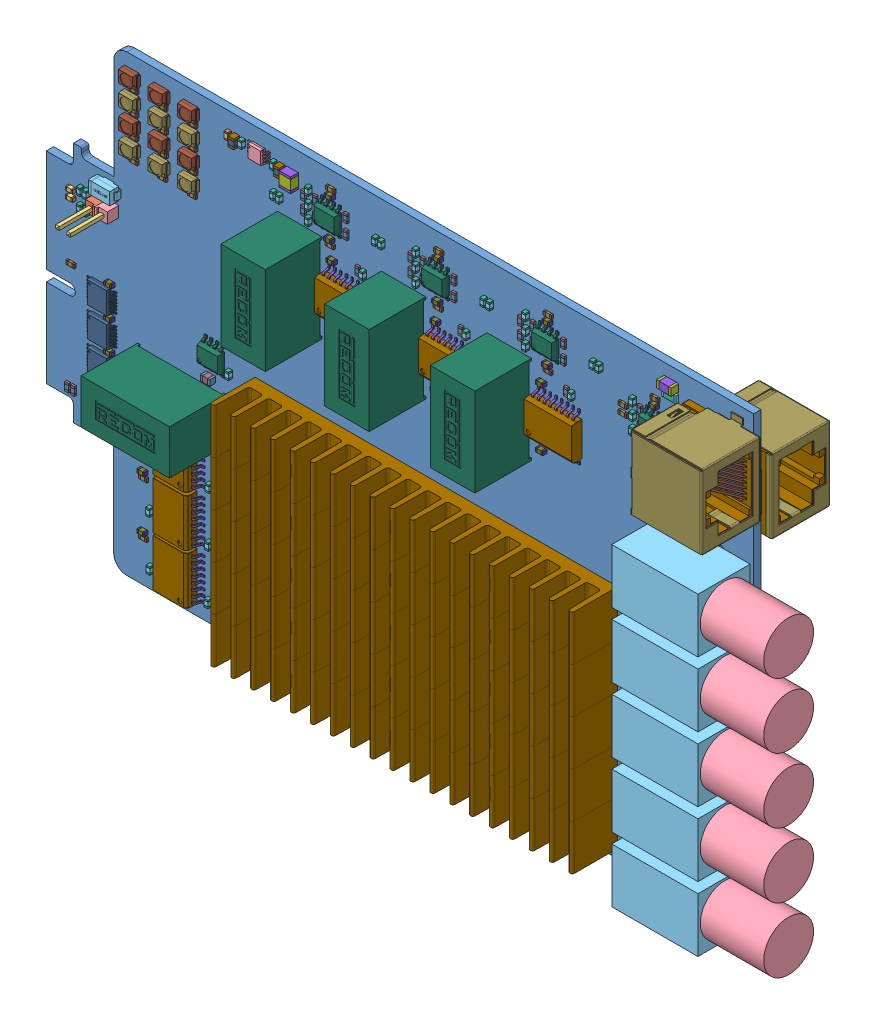
SolidWorks assembly 1166V10, configuration Standard. Lengths in mm. (continued)
Components (placement in the parent): (continued)
- 1166V10.step-1: 1166V10.step [Standard] at origin size (170.01 100 28.53) (continued)
  - R419.step-1: R419.step [Standard] at origin size (0.85 1.85 0.45) (continued)
    - 6549605008.step-1: 6549605008.step [Standard] at (66.31 93.45 0) size (0.85 0.45 0.45) (continued)
      - Extruded-7.step-1: Extruded-7.step [Standard] at origin size (0.85 0.45 0.45)
    - 6549605008.step-2: 6549605008.step [Standard] at (66.31 92.05 0) size (0.85 0.45 0.45)
      - Extruded-7.step-1: Extruded-7.step [Standard] at origin size (0.85 0.45 0.45)
    - 6549605488.step-1: 6549605488.step [Standard] at (66.31 92.75 0) size (0.85 0.95 0.45)
      - Extruded-8.step-1: Extruded-8.step [Standard] at origin size (0.85 0.95 0.45)
  - R418.step-1: R418.step [Standard] at origin size (1.85 0.85 0.45)
    - 6547171712.step-1: 6547171712.step [Standard] at (62.26 96.5 0) size (0.45 0.85 0.45)
      - Extruded-5.step-1: Extruded-5.step [Standard] at origin size (0.45 0.85 0.45)
    - 6547171712.step-2: 6547171712.step [Standard] at (63.66 96.5 0) size (0.45 0.85 0.45)
      - Extruded-5.step-1: Extruded-5.step [Standard] at origin size (0.45 0.85 0.45)
    - 6547171152.step-1: 6547171152.step [Standard] at (62.96 96.5 0) size (0.95 0.85 0.45)
      - Extruded-6.step-1: Extruded-6.step [Standard] at origin size (0.95 0.85 0.45)
  - R416.step-1: R416.step [Standard] at origin size (1.85 0.85 0.45)
    - 6547171712.step-1: 6547171712.step [Standard] at (22.35 31.8 0) size (0.45 0.85 0.45)
      - Extruded-5.step-1: Extruded-5.step [Standard] at origin size (0.45 0.85 0.45)
    - 6547171712.step-2: 6547171712.step [Standard] at (20.95 31.8 0) size (0.45 0.85 0.45)
      - Extruded-5.step-1: Extruded-5.step [Standard] at origin size (0.45 0.85 0.45)
    - 6547171152.step-1: 6547171152.step [Standard] at (21.65 31.8 0) size (0.95 0.85 0.45)
      - Extruded-6.step-1: Extruded-6.step [Standard] at origin size (0.95 0.85 0.45)
  - R413.step-1: R413.step [Standard] at origin size (0.85 1.85 0.45)
    - 6549605008.step-1: 6549605008.step [Standard] at (68.9 83.25 0) size (0.85 0.45 0.45)
      - Extruded-7.step-1: Extruded-7.step [Standard] at origin size (0.85 0.45 0.45)
    - 6549605008.step-2: 6549605008.step [Standard] at (68.9 84.65 0) size (0.85 0.45 0.45)
      - Extruded-7.step-1: Extruded-7.step [Standard] at origin size (0.85 0.45 0.45)
    - 6549605488.step-1: 6549605488.step [Standard] at (68.9 83.95 0) size (0.85 0.95 0.45)
      - Extruded-8.step-1: Extruded-8.step [Standard] at origin size (0.85 0.95 0.45)
  - R325.step-1: R325.step [Standard] at origin size (1.85 0.85 0.45)
    - 6547171712.step-1: 6547171712.step [Standard] at (85.96 85.8 0) size (0.45 0.85 0.45)
      - Extruded-5.step-1: Extruded-5.step [Standard] at origin size (0.45 0.85 0.45)
    - 6547171712.step-2: 6547171712.step [Standard] at (87.36 85.8 0) size (0.45 0.85 0.45)
      - Extruded-5.step-1: Extruded-5.step [Standard] at origin size (0.45 0.85 0.45)
    - 6547171152.step-1: 6547171152.step [Standard] at (86.66 85.8 0) size (0.95 0.85 0.45)
      - Extruded-6.step-1: Extruded-6.step [Standard] at origin size (0.95 0.85 0.45)
  - R324.step-1: R324.step [Standard] at origin size (0.85 1.85 0.45)
    - 6549605008.step-1: 6549605008.step [Standard] at (80.61 88.75 0) size (0.85 0.45 0.45)
      - Extruded-7.step-1: Extruded-7.step [Standard] at origin size (0.85 0.45 0.45)
    - 6549605008.step-2: 6549605008.step [Standard] at (80.61 90.15 0) size (0.85 0.45 0.45)
      - Extruded-7.step-1: Extruded-7.step [Standard] at origin size (0.85 0.45 0.45)
    - 6549605488.step-1: 6549605488.step [Standard] at (80.61 89.45 0) size (0.85 0.95 0.45)
      - Extruded-8.step-1: Extruded-8.step [Standard] at origin size (0.85 0.95 0.45)
  - R323.step-1: R323.step [Standard] at origin size (0.85 1.85 0.45)
    - 6549605008.step-1: 6549605008.step [Standard] at (83.31 90.25 0) size (0.85 0.45 0.45)
      - Extruded-7.step-1: Extruded-7.step [Standard] at origin size (0.85 0.45 0.45)
    - 6549605008.step-2: 6549605008.step [Standard] at (83.31 88.85 0) size (0.85 0.45 0.45)
      - Extruded-7.step-1: Extruded-7.step [Standard] at origin size (0.85 0.45 0.45)
    - 6549605488.step-1: 6549605488.step [Standard] at (83.31 89.55 0) size (0.85 0.95 0.45)
      - Extruded-8.step-1: Extruded-8.step [Standard] at origin size (0.85 0.95 0.45)
  - R322.step-1: R322.step [Standard] at origin size (0.85 1.85 0.45)
    - 6549605008.step-1: 6549605008.step [Standard] at (90.11 88.85 0) size (0.85 0.45 0.45)
      - Extruded-7.step-1: Extruded-7.step [Standard] at origin size (0.85 0.45 0.45)
    - 6549605008.step-2: 6549605008.step [Standard] at (90.11 90.25 0) size (0.85 0.45 0.45)
      - Extruded-7.step-1: Extruded-7.step [Standard] at origin size (0.85 0.45 0.45)
    - 6549605488.step-1: 6549605488.step [Standard] at (90.11 89.55 0) size (0.85 0.95 0.45)
      - Extruded-8.step-1: Extruded-8.step [Standard] at origin size (0.85 0.95 0.45)
  - R321.step-1: R321.step [Standard] at origin size (0.85 1.85 0.45)
    - 6549605008.step-1: 6549605008.step [Standard] at (80.61 91.65 0) size (0.85 0.45 0.45)
      - Extruded-7.step-1: Extruded-7.step [Standard] at origin size (0.85 0.45 0.45)
    - 6549605008.step-2: 6549605008.step [Standard] at (80.61 93.05 0) size (0.85 0.45 0.45)
      - Extruded-7.step-1: Extruded-7.step [Standard] at origin size (0.85 0.45 0.45)
    - 6549605488.step-1: 6549605488.step [Standard] at (80.61 92.35 0) size (0.85 0.95 0.45)
      - Extruded-8.step-1: Extruded-8.step [Standard] at origin size (0.85 0.95 0.45)
  - R320.step-1: R320.step [Standard] at origin size (0.85 1.85 0.45)
    - 6549605008.step-1: 6549605008.step [Standard] at (83.31 92.05 0) size (0.85 0.45 0.45)
      - Extruded-7.step-1: Extruded-7.step [Standard] at origin size (0.85 0.45 0.45)
    - 6549605008.step-2: 6549605008.step [Standard] at (83.31 93.45 0) size (0.85 0.45 0.45)
      - Extruded-7.step-1: Extruded-7.step [Standard] at origin size (0.85 0.45 0.45)
    - 6549605488.step-1: 6549605488.step [Standard] at (83.31 92.75 0) size (0.85 0.95 0.45)
      - Extruded-8.step-1: Extruded-8.step [Standard] at origin size (0.85 0.95 0.45)
  - R319.step-1: R319.step [Standard] at origin size (0.85 1.85 0.45)
    - 6549605008.step-1: 6549605008.step [Standard] at (90.11 93.45 0) size (0.85 0.45 0.45)
      - Extruded-7.step-1: Extruded-7.step [Standard] at origin size (0.85 0.45 0.45)
    - 6549605008.step-2: 6549605008.step [Standard] at (90.11 92.05 0) size (0.85 0.45 0.45)
      - Extruded-7.step-1: Extruded-7.step [Standard] at origin size (0.85 0.45 0.45)
    - 6549605488.step-1: 6549605488.step [Standard] at (90.11 92.75 0) size (0.85 0.95 0.45)
      - Extruded-8.step-1: Extruded-8.step [Standard] at origin size (0.85 0.95 0.45)
  - R318.step-1: R318.step [Standard] at origin size (1.85 0.85 0.45)
    - 6547171712.step-1: 6547171712.step [Standard] at (86.06 96.5 0) size (0.45 0.85 0.45)
      - Extruded-5.step-1: Extruded-5.step [Standard] at origin size (0.45 0.85 0.45)
    - 6547171712.step-2: 6547171712.step [Standard] at (87.46 96.5 0) size (0.45 0.85 0.45)
      - Extruded-5.step-1: Extruded-5.step [Standard] at origin size (0.45 0.85 0.45)
    - 6547171152.step-1: 6547171152.step [Standard] at (86.76 96.5 0) size (0.95 0.85 0.45)
      - Extruded-6.step-1: Extruded-6.step [Standard] at origin size (0.95 0.85 0.45)
  - R316.step-1: R316.step [Standard] at origin size (1.85 0.85 0.45)
    - 6547171712.step-1: 6547171712.step [Standard] at (22.35 20.7 0) size (0.45 0.85 0.45)
      - Extruded-5.step-1: Extruded-5.step [Standard] at origin size (0.45 0.85 0.45)
    - 6547171712.step-2: 6547171712.step [Standard] at (20.95 20.7 0) size (0.45 0.85 0.45)
      - Extruded-5.step-1: Extruded-5.step [Standard] at origin size (0.45 0.85 0.45)
    - 6547171152.step-1: 6547171152.step [Standard] at (21.65 20.7 0) size (0.95 0.85 0.45)
      - Extruded-6.step-1: Extruded-6.step [Standard] at origin size (0.95 0.85 0.45)
  - R313.step-1: R313.step [Standard] at origin size (0.85 1.85 0.45)
    - 6549605008.step-1: 6549605008.step [Standard] at (91.7 83.15 0) size (0.85 0.45 0.45)
      - Extruded-7.step-1: Extruded-7.step [Standard] at origin size (0.85 0.45 0.45)
    - 6549605008.step-2: 6549605008.step [Standard] at (91.7 84.55 0) size (0.85 0.45 0.45)
      - Extruded-7.step-1: Extruded-7.step [Standard] at origin size (0.85 0.45 0.45)
    - 6549605488.step-1: 6549605488.step [Standard] at (91.7 83.85 0) size (0.85 0.95 0.45)
      - Extruded-8.step-1: Extruded-8.step [Standard] at origin size (0.85 0.95 0.45)
  - R225.step-1: R225.step [Standard] at origin size (1.85 0.85 0.45)
    - 6547171712.step-1: 6547171712.step [Standard] at (110.15 85.8 0) size (0.45 0.85 0.45)
      - Extruded-5.step-1: Extruded-5.step [Standard] at origin size (0.45 0.85 0.45)
    - 6547171712.step-2: 6547171712.step [Standard] at (111.55 85.8 0) size (0.45 0.85 0.45)
      - Extruded-5.step-1: Extruded-5.step [Standard] at origin size (0.45 0.85 0.45)
    - 6547171152.step-1: 6547171152.step [Standard] at (110.85 85.8 0) size (0.95 0.85 0.45)
      - Extruded-6.step-1: Extruded-6.step [Standard] at origin size (0.95 0.85 0.45)
  - R224.step-1: R224.step [Standard] at origin size (0.85 1.85 0.45)
    - 6549605008.step-1: 6549605008.step [Standard] at (107.5 90.25 0) size (0.85 0.45 0.45)
      - Extruded-7.step-1: Extruded-7.step [Standard] at origin size (0.85 0.45 0.45)
    - 6549605008.step-2: 6549605008.step [Standard] at (107.5 88.85 0) size (0.85 0.45 0.45)
      - Extruded-7.step-1: Extruded-7.step [Standard] at origin size (0.85 0.45 0.45)
    - 6549605488.step-1: 6549605488.step [Standard] at (107.5 89.55 0) size (0.85 0.95 0.45)
      - Extruded-8.step-1: Extruded-8.step [Standard] at origin size (0.85 0.95 0.45)
  - R223.step-1: R223.step [Standard] at origin size (0.85 1.85 0.45)
    - 6549605008.step-1: 6549605008.step [Standard] at (114.3 88.85 0) size (0.85 0.45 0.45)
      - Extruded-7.step-1: Extruded-7.step [Standard] at origin size (0.85 0.45 0.45)
    - 6549605008.step-2: 6549605008.step [Standard] at (114.3 90.25 0) size (0.85 0.45 0.45)
      - Extruded-7.step-1: Extruded-7.step [Standard] at origin size (0.85 0.45 0.45)
    - 6549605488.step-1: 6549605488.step [Standard] at (114.3 89.55 0) size (0.85 0.95 0.45)
      - Extruded-8.step-1: Extruded-8.step [Standard] at origin size (0.85 0.95 0.45)
  - R222.step-1: R222.step [Standard] at origin size (0.85 1.85 0.45)
    - 6549605008.step-1: 6549605008.step [Standard] at (107.5 92.05 0) size (0.85 0.45 0.45)
      - Extruded-7.step-1: Extruded-7.step [Standard] at origin size (0.85 0.45 0.45)
    - 6549605008.step-2: 6549605008.step [Standard] at (107.5 93.45 0) size (0.85 0.45 0.45)
      - Extruded-7.step-1: Extruded-7.step [Standard] at origin size (0.85 0.45 0.45)
    - 6549605488.step-1: 6549605488.step [Standard] at (107.5 92.75 0) size (0.85 0.95 0.45)
      - Extruded-8.step-1: Extruded-8.step [Standard] at origin size (0.85 0.95 0.45)
  - R221.step-1: R221.step [Standard] at origin size (0.85 1.85 0.45)
    - 6549605008.step-1: 6549605008.step [Standard] at (114.3 93.45 0) size (0.85 0.45 0.45)
      - Extruded-7.step-1: Extruded-7.step [Standard] at origin size (0.85 0.45 0.45)
    - 6549605008.step-2: 6549605008.step [Standard] at (114.3 92.05 0) size (0.85 0.45 0.45)
      - Extruded-7.step-1: Extruded-7.step [Standard] at origin size (0.85 0.45 0.45)
    - 6549605488.step-1: 6549605488.step [Standard] at (114.3 92.75 0) size (0.85 0.95 0.45)
      - Extruded-8.step-1: Extruded-8.step [Standard] at origin size (0.85 0.95 0.45)
  - R220.step-1: R220.step [Standard] at origin size (1.85 0.85 0.45)
    - 6547171712.step-1: 6547171712.step [Standard] at (110.25 96.5 0) size (0.45 0.85 0.45)
      - Extruded-5.step-1: Extruded-5.step [Standard] at origin size (0.45 0.85 0.45)
    - 6547171712.step-2: 6547171712.step [Standard] at (111.65 96.5 0) size (0.45 0.85 0.45)
      - Extruded-5.step-1: Extruded-5.step [Standard] at origin size (0.45 0.85 0.45)
    - 6547171152.step-1: 6547171152.step [Standard] at (110.95 96.5 0) size (0.95 0.85 0.45)
      - Extruded-6.step-1: Extruded-6.step [Standard] at origin size (0.95 0.85 0.45)
  - R219.step-1: R219.step [Standard] at origin size (1.85 0.85 0.45)
    - 6547171712.step-1: 6547171712.step [Standard] at (22.35 9.3 0) size (0.45 0.85 0.45)
      - Extruded-5.step-1: Extruded-5.step [Standard] at origin size (0.45 0.85 0.45)
    - 6547171712.step-2: 6547171712.step [Standard] at (20.95 9.3 0) size (0.45 0.85 0.45)
      - Extruded-5.step-1: Extruded-5.step [Standard] at origin size (0.45 0.85 0.45)
    - 6547171152.step-1: 6547171152.step [Standard] at (21.65 9.3 0) size (0.95 0.85 0.45)
      - Extruded-6.step-1: Extruded-6.step [Standard] at origin size (0.95 0.85 0.45)
  - R218.step-1: R218.step [Standard] at origin size (0.85 1.85 0.45)
    - 6549605008.step-1: 6549605008.step [Standard] at (114.9 83.15 0) size (0.85 0.45 0.45)
      - Extruded-7.step-1: Extruded-7.step [Standard] at origin size (0.85 0.45 0.45)
    - 6549605008.step-2: 6549605008.step [Standard] at (114.9 84.55 0) size (0.85 0.45 0.45)
      - Extruded-7.step-1: Extruded-7.step [Standard] at origin size (0.85 0.45 0.45)
    - 6549605488.step-1: 6549605488.step [Standard] at (114.9 83.85 0) size (0.85 0.95 0.45)
      - Extruded-8.step-1: Extruded-8.step [Standard] at origin size (0.85 0.95 0.45)
  - IC507.step-1: IC507.step [Standard] at origin size (4.83 6.2 1.7)
    - SOIC-8_Narrow.step-1: SOIC-8_Narrow.step [Standard] at (95.6301 91.2361 -1.622) x (-1 0 0) z (0 -1 0) size (4.83 1.7 6.2)
  - IC506.step-1: IC506.step [Standard] at origin size (4.83 6.2 1.7)
    - SOIC-8_Narrow.step-1: SOIC-8_Narrow.step [Standard] at (71.7901 90.9361 -1.622) x (-1 0 0) z (0 -1 0) size (4.83 1.7 6.2)
  - IC505.step-1: IC505.step [Standard] at origin size (4.83 6.2 1.7)
    - SOIC-8_Narrow.step-1: SOIC-8_Narrow.step [Standard] at (119.8001 91.3361 -1.622) x (-1 0 0) z (0 -1 0) size (4.83 1.7 6.2)
  - IC504.step-1: IC504.step [Standard] at origin size (4.83 6.2 1.7)
    - SOIC-8_Narrow.step-1: SOIC-8_Narrow.step [Standard] at (49.2601 88.4361 -1.622) x (-1 0 0) z (0 -1 0) size (4.83 1.7 6.2)
  - IC503.step-1: IC503.step [Standard] at origin size (4.83 6.2 1.7)
    - SOIC-8_Narrow.step-1: SOIC-8_Narrow.step [Standard] at (132.5901 86.8639 0) x (-1 0 0) z (0 1 0) size (4.83 1.7 6.2)
  - IC405.step-1: IC405.step [Standard] at origin size (4.83 6.2 1.7)
    - SOIC-8_Narrow.step-1: SOIC-8_Narrow.step [Standard] at (61.0001 91.1639 0) x (-1 0 0) z (0 1 0) size (4.83 1.7 6.2)
  - IC305.step-1: IC305.step [Standard] at origin size (4.83 6.2 1.7)
    - SOIC-8_Narrow.step-1: SOIC-8_Narrow.step [Standard] at (84.8001 91.1639 0) x (-1 0 0) z (0 1 0) size (4.83 1.7 6.2)
  - IC206.step-1: IC206.step [Standard] at origin size (4.83 6.2 1.7)
    - SOIC-8_Narrow.step-1: SOIC-8_Narrow.step [Standard] at (108.9901 91.1639 0) x (-1 0 0) z (0 1 0) size (4.83 1.7 6.2)
  - C539.step-1: C539.step [Standard] at origin size (1.6 0.82 0.9)
    - 6547664352.step-1: 6547664352.step [Standard] at (97.65 95.4 -2.522) size (0.9 0.82 0.9)
      - Extruded-9.step-1: Extruded-9.step [Standard] at origin size (0.9 0.82 0.9)
    - 6547664912.step-1: 6547664912.step [Standard] at (98.275 95.4 -2.522) size (0.35 0.82 0.9)
      - Extruded-10.step-1: Extruded-10.step [Standard] at origin size (0.35 0.82 0.9)
    - 6547664912.step-2: 6547664912.step [Standard] at (97.025 95.4 -2.522) size (0.35 0.82 0.9)
      - Extruded-10.step-1: Extruded-10.step [Standard] at origin size (0.35 0.82 0.9)
  - C538.step-1: C538.step [Standard] at origin size (0.82 1.6 0.9)
    - 6547668352.step-1: 6547668352.step [Standard] at (92.7 94.05 -2.522) size (0.82 0.9 0.9)
      - Extruded.step-1: Extruded.step [Standard] at origin size (0.82 0.9 0.9)
    - 6549602528.step-1: 6549602528.step [Standard] at (92.7 93.425 -2.522) size (0.82 0.35 0.9)
      - Extruded-0.step-1: Extruded-0.step [Standard] at origin size (0.82 0.35 0.9)
    - 6549602528.step-2: 6549602528.step [Standard] at (92.7 94.675 -2.522) size (0.82 0.35 0.9)
      - Extruded-0.step-1: Extruded-0.step [Standard] at origin size (0.82 0.35 0.9)
  - C537.step-1: C537.step [Standard] at origin size (0.82 1.6 0.9)
    - 6547668352.step-1: 6547668352.step [Standard] at (92.7 91.25 -2.522) size (0.82 0.9 0.9)
      - Extruded.step-1: Extruded.step [Standard] at origin size (0.82 0.9 0.9)
    - 6549602528.step-1: 6549602528.step [Standard] at (92.7 90.625 -2.522) size (0.82 0.35 0.9)
      - Extruded-0.step-1: Extruded-0.step [Standard] at origin size (0.82 0.35 0.9)
    - 6549602528.step-2: 6549602528.step [Standard] at (92.7 91.875 -2.522) size (0.82 0.35 0.9)
      - Extruded-0.step-1: Extruded-0.step [Standard] at origin size (0.82 0.35 0.9)
  - C536.step-1: C536.step [Standard] at origin size (0.82 1.6 0.9)
    - 6547668352.step-1: 6547668352.step [Standard] at (92.7 88.45 -2.522) size (0.82 0.9 0.9)
      - Extruded.step-1: Extruded.step [Standard] at origin size (0.82 0.9 0.9)
    - 6549602528.step-1: 6549602528.step [Standard] at (92.7 87.825 -2.522) size (0.82 0.35 0.9)
      - Extruded-0.step-1: Extruded-0.step [Standard] at origin size (0.82 0.35 0.9)
    - 6549602528.step-2: 6549602528.step [Standard] at (92.7 89.075 -2.522) size (0.82 0.35 0.9)
      - Extruded-0.step-1: Extruded-0.step [Standard] at origin size (0.82 0.35 0.9)
  - C535.step-1: C535.step [Standard] at origin size (1.6 0.82 0.9)
    - 6547664352.step-1: 6547664352.step [Standard] at (97.55 87.1 -2.522) size (0.9 0.82 0.9)
      - Extruded-9.step-1: Extruded-9.step [Standard] at origin size (0.9 0.82 0.9)
    - 6547664912.step-1: 6547664912.step [Standard] at (98.175 87.1 -2.522) size (0.35 0.82 0.9)
      - Extruded-10.step-1: Extruded-10.step [Standard] at origin size (0.35 0.82 0.9)
    - 6547664912.step-2: 6547664912.step [Standard] at (96.925 87.1 -2.522) size (0.35 0.82 0.9)
      - Extruded-10.step-1: Extruded-10.step [Standard] at origin size (0.35 0.82 0.9)
  - C534.step-1: C534.step [Standard] at origin size (1.6 0.82 0.9)
    - 6547664352.step-1: 6547664352.step [Standard] at (73.75 95.1 -2.522) size (0.9 0.82 0.9)
      - Extruded-9.step-1: Extruded-9.step [Standard] at origin size (0.9 0.82 0.9)
    - 6547664912.step-1: 6547664912.step [Standard] at (74.375 95.1 -2.522) size (0.35 0.82 0.9)
      - Extruded-10.step-1: Extruded-10.step [Standard] at origin size (0.35 0.82 0.9)
    - 6547664912.step-2: 6547664912.step [Standard] at (73.125 95.1 -2.522) size (0.35 0.82 0.9)
      - Extruded-10.step-1: Extruded-10.step [Standard] at origin size (0.35 0.82 0.9)
  - C533.step-1: C533.step [Standard] at origin size (0.82 1.6 0.9)
    - 6547668352.step-1: 6547668352.step [Standard] at (68.9 93.75 -2.522) size (0.82 0.9 0.9)
      - Extruded.step-1: Extruded.step [Standard] at origin size (0.82 0.9 0.9)
    - 6549602528.step-1: 6549602528.step [Standard] at (68.9 93.125 -2.522) size (0.82 0.35 0.9)
      - Extruded-0.step-1: Extruded-0.step [Standard] at origin size (0.82 0.35 0.9)
    - 6549602528.step-2: 6549602528.step [Standard] at (68.9 94.375 -2.522) size (0.82 0.35 0.9)
      - Extruded-0.step-1: Extruded-0.step [Standard] at origin size (0.82 0.35 0.9)
  - C532.step-1: C532.step [Standard] at origin size (0.82 1.6 0.9)
    - 6547668352.step-1: 6547668352.step [Standard] at (68.9 90.95 -2.522) size (0.82 0.9 0.9)
      - Extruded.step-1: Extruded.step [Standard] at origin size (0.82 0.9 0.9)
    - 6549602528.step-1: 6549602528.step [Standard] at (68.9 90.325 -2.522) size (0.82 0.35 0.9)
      - Extruded-0.step-1: Extruded-0.step [Standard] at origin size (0.82 0.35 0.9)
    - 6549602528.step-2: 6549602528.step [Standard] at (68.9 91.575 -2.522) size (0.82 0.35 0.9)
      - Extruded-0.step-1: Extruded-0.step [Standard] at origin size (0.82 0.35 0.9)
  - C531.step-1: C531.step [Standard] at origin size (0.82 1.6 0.9)
    - 6547668352.step-1: 6547668352.step [Standard] at (68.9 88.15 -2.522) size (0.82 0.9 0.9)
      - Extruded.step-1: Extruded.step [Standard] at origin size (0.82 0.9 0.9)
    - 6549602528.step-1: 6549602528.step [Standard] at (68.9 87.525 -2.522) size (0.82 0.35 0.9)
      - Extruded-0.step-1: Extruded-0.step [Standard] at origin size (0.82 0.35 0.9)
    - 6549602528.step-2: 6549602528.step [Standard] at (68.9 88.775 -2.522) size (0.82 0.35 0.9)
      - Extruded-0.step-1: Extruded-0.step [Standard] at origin size (0.82 0.35 0.9)
  - C530.step-1: C530.step [Standard] at origin size (1.6 0.82 0.9)
    - 6547664352.step-1: 6547664352.step [Standard] at (121.75 95.5 -2.522) size (0.9 0.82 0.9)
      - Extruded-9.step-1: Extruded-9.step [Standard] at origin size (0.9 0.82 0.9)
    - 6547664912.step-1: 6547664912.step [Standard] at (122.375 95.5 -2.522) size (0.35 0.82 0.9)
      - Extruded-10.step-1: Extruded-10.step [Standard] at origin size (0.35 0.82 0.9)
    - 6547664912.step-2: 6547664912.step [Standard] at (121.125 95.5 -2.522) size (0.35 0.82 0.9)
      - Extruded-10.step-1: Extruded-10.step [Standard] at origin size (0.35 0.82 0.9)
  - C529.step-1: C529.step [Standard] at origin size (0.82 1.6 0.9)
    - 6547668352.step-1: 6547668352.step [Standard] at (116.9 94.45 -2.522) size (0.82 0.9 0.9)
      - Extruded.step-1: Extruded.step [Standard] at origin size (0.82 0.9 0.9)
    - 6549602528.step-1: 6549602528.step [Standard] at (116.9 93.825 -2.522) size (0.82 0.35 0.9)
      - Extruded-0.step-1: Extruded-0.step [Standard] at origin size (0.82 0.35 0.9)
    - 6549602528.step-2: 6549602528.step [Standard] at (116.9 95.075 -2.522) size (0.82 0.35 0.9)
      - Extruded-0.step-1: Extruded-0.step [Standard] at origin size (0.82 0.35 0.9)
  - C528.step-1: C528.step [Standard] at origin size (1.6 0.82 0.9)
    - 6547664352.step-1: 6547664352.step [Standard] at (73.75 86.8 -2.522) size (0.9 0.82 0.9)
      - Extruded-9.step-1: Extruded-9.step [Standard] at origin size (0.9 0.82 0.9)
    - 6547664912.step-1: 6547664912.step [Standard] at (74.375 86.8 -2.522) size (0.35 0.82 0.9)
      - Extruded-10.step-1: Extruded-10.step [Standard] at origin size (0.35 0.82 0.9)
    - 6547664912.step-2: 6547664912.step [Standard] at (73.125 86.8 -2.522) size (0.35 0.82 0.9)
      - Extruded-10.step-1: Extruded-10.step [Standard] at origin size (0.35 0.82 0.9)
  - C527.step-1: C527.step [Standard] at origin size (0.82 1.6 0.9)
    - 6547668352.step-1: 6547668352.step [Standard] at (116.9 91.65 -2.522) size (0.82 0.9 0.9)
      - Extruded.step-1: Extruded.step [Standard] at origin size (0.82 0.9 0.9)
    - 6549602528.step-1: 6549602528.step [Standard] at (116.9 91.025 -2.522) size (0.82 0.35 0.9)
      - Extruded-0.step-1: Extruded-0.step [Standard] at origin size (0.82 0.35 0.9)
    - 6549602528.step-2: 6549602528.step [Standard] at (116.9 92.275 -2.522) size (0.82 0.35 0.9)
      - Extruded-0.step-1: Extruded-0.step [Standard] at origin size (0.82 0.35 0.9)
  - C526.step-1: C526.step [Standard] at origin size (0.82 1.6 0.9)
    - 6547668352.step-1: 6547668352.step [Standard] at (116.9 88.85 -2.522) size (0.82 0.9 0.9)
      - Extruded.step-1: Extruded.step [Standard] at origin size (0.82 0.9 0.9)
    - 6549602528.step-1: 6549602528.step [Standard] at (116.9 88.225 -2.522) size (0.82 0.35 0.9)
      - Extruded-0.step-1: Extruded-0.step [Standard] at origin size (0.82 0.35 0.9)
    - 6549602528.step-2: 6549602528.step [Standard] at (116.9 89.475 -2.522) size (0.82 0.35 0.9)
      - Extruded-0.step-1: Extruded-0.step [Standard] at origin size (0.82 0.35 0.9)
  - C525.step-1: C525.step [Standard] at origin size (1.6 0.82 0.9)
    - 6547664352.step-1: 6547664352.step [Standard] at (121.65 87.2 -2.522) size (0.9 0.82 0.9)
      - Extruded-9.step-1: Extruded-9.step [Standard] at origin size (0.9 0.82 0.9)
    - 6547664912.step-1: 6547664912.step [Standard] at (122.275 87.2 -2.522) size (0.35 0.82 0.9)
      - Extruded-10.step-1: Extruded-10.step [Standard] at origin size (0.35 0.82 0.9)
    - 6547664912.step-2: 6547664912.step [Standard] at (121.025 87.2 -2.522) size (0.35 0.82 0.9)
      - Extruded-10.step-1: Extruded-10.step [Standard] at origin size (0.35 0.82 0.9)
  - C524.step-1: C524.step [Standard] at origin size (1.6 0.82 0.9)
    - 6547664352.step-1: 6547664352.step [Standard] at (51.15 92.6 -2.522) size (0.9 0.82 0.9)
      - Extruded-9.step-1: Extruded-9.step [Standard] at origin size (0.9 0.82 0.9)
    - 6547664912.step-1: 6547664912.step [Standard] at (51.775 92.6 -2.522) size (0.35 0.82 0.9)
      - Extruded-10.step-1: Extruded-10.step [Standard] at origin size (0.35 0.82 0.9)
    - 6547664912.step-2: 6547664912.step [Standard] at (50.525 92.6 -2.522) size (0.35 0.82 0.9)
      - Extruded-10.step-1: Extruded-10.step [Standard] at origin size (0.35 0.82 0.9)
  - C523.step-1: C523.step [Standard] at origin size (0.82 1.6 0.9)
    - 6547668352.step-1: 6547668352.step [Standard] at (46.3 91.35 -2.522) size (0.82 0.9 0.9)
      - Extruded.step-1: Extruded.step [Standard] at origin size (0.82 0.9 0.9)
    - 6549602528.step-1: 6549602528.step [Standard] at (46.3 90.725 -2.522) size (0.82 0.35 0.9)
      - Extruded-0.step-1: Extruded-0.step [Standard] at origin size (0.82 0.35 0.9)
    - 6549602528.step-2: 6549602528.step [Standard] at (46.3 91.975 -2.522) size (0.82 0.35 0.9)
      - Extruded-0.step-1: Extruded-0.step [Standard] at origin size (0.82 0.35 0.9)
  - C522.step-1: C522.step [Standard] at origin size (0.82 1.6 0.9)
    - 6547668352.step-1: 6547668352.step [Standard] at (46.3 88.55 -2.522) size (0.82 0.9 0.9)
      - Extruded.step-1: Extruded.step [Standard] at origin size (0.82 0.9 0.9)
    - 6549602528.step-1: 6549602528.step [Standard] at (46.3 87.925 -2.522) size (0.82 0.35 0.9)
      - Extruded-0.step-1: Extruded-0.step [Standard] at origin size (0.82 0.35 0.9)
    - 6549602528.step-2: 6549602528.step [Standard] at (46.3 89.175 -2.522) size (0.82 0.35 0.9)
      - Extruded-0.step-1: Extruded-0.step [Standard] at origin size (0.82 0.35 0.9)
  - C521.step-1: C521.step [Standard] at origin size (0.82 1.6 0.9)
    - 6547668352.step-1: 6547668352.step [Standard] at (46.3 85.75 -2.522) size (0.82 0.9 0.9)
      - Extruded.step-1: Extruded.step [Standard] at origin size (0.82 0.9 0.9)
    - 6549602528.step-1: 6549602528.step [Standard] at (46.3 85.125 -2.522) size (0.82 0.35 0.9)
      - Extruded-0.step-1: Extruded-0.step [Standard] at origin size (0.82 0.35 0.9)
    - 6549602528.step-2: 6549602528.step [Standard] at (46.3 86.375 -2.522) size (0.82 0.35 0.9)
      - Extruded-0.step-1: Extruded-0.step [Standard] at origin size (0.82 0.35 0.9)
  - C520.step-1: C520.step [Standard] at origin size (1.6 0.82 0.9)
    - 6547664352.step-1: 6547664352.step [Standard] at (51.15 84.3 -2.522) size (0.9 0.82 0.9)
      - Extruded-9.step-1: Extruded-9.step [Standard] at origin size (0.9 0.82 0.9)
    - 6547664912.step-1: 6547664912.step [Standard] at (51.775 84.3 -2.522) size (0.35 0.82 0.9)
      - Extruded-10.step-1: Extruded-10.step [Standard] at origin size (0.35 0.82 0.9)
    - 6547664912.step-2: 6547664912.step [Standard] at (50.525 84.3 -2.522) size (0.35 0.82 0.9)
      - Extruded-10.step-1: Extruded-10.step [Standard] at origin size (0.35 0.82 0.9)
  - C519.step-1: C519.step [Standard] at origin size (1.6 0.82 0.9)
    - 6547664352.step-1: 6547664352.step [Standard] at (134.45 82.6 0) size (0.9 0.82 0.9)
      - Extruded-9.step-1: Extruded-9.step [Standard] at origin size (0.9 0.82 0.9)
    - 6547664912.step-1: 6547664912.step [Standard] at (135.075 82.6 0) size (0.35 0.82 0.9)
      - Extruded-10.step-1: Extruded-10.step [Standard] at origin size (0.35 0.82 0.9)
    - 6547664912.step-2: 6547664912.step [Standard] at (133.825 82.6 0) size (0.35 0.82 0.9)
      - Extruded-10.step-1: Extruded-10.step [Standard] at origin size (0.35 0.82 0.9)
  - C518.step-1: C518.step [Standard] at origin size (0.82 1.6 0.9)
    - 6547668352.step-1: 6547668352.step [Standard] at (129.7 83.95 0) size (0.82 0.9 0.9)
      - Extruded.step-1: Extruded.step [Standard] at origin size (0.82 0.9 0.9)
    - 6549602528.step-1: 6549602528.step [Standard] at (129.7 84.575 0) size (0.82 0.35 0.9)
      - Extruded-0.step-1: Extruded-0.step [Standard] at origin size (0.82 0.35 0.9)
    - 6549602528.step-2: 6549602528.step [Standard] at (129.7 83.325 0) size (0.82 0.35 0.9)
      - Extruded-0.step-1: Extruded-0.step [Standard] at origin size (0.82 0.35 0.9)
  - C516.step-1: C516.step [Standard] at origin size (0.82 1.6 0.9)
    - 6547668352.step-1: 6547668352.step [Standard] at (129.7 86.75 0) size (0.82 0.9 0.9)
      - Extruded.step-1: Extruded.step [Standard] at origin size (0.82 0.9 0.9)
    - 6549602528.step-1: 6549602528.step [Standard] at (129.7 87.375 0) size (0.82 0.35 0.9)
      - Extruded-0.step-1: Extruded-0.step [Standard] at origin size (0.82 0.35 0.9)
    - 6549602528.step-2: 6549602528.step [Standard] at (129.7 86.125 0) size (0.82 0.35 0.9)
      - Extruded-0.step-1: Extruded-0.step [Standard] at origin size (0.82 0.35 0.9)
  - C512.step-1: C512.step [Standard] at origin size (0.82 1.6 0.9)
    - 6547668352.step-1: 6547668352.step [Standard] at (129.7 89.55 0) size (0.82 0.9 0.9)
      - Extruded.step-1: Extruded.step [Standard] at origin size (0.82 0.9 0.9)
    - 6549602528.step-1: 6549602528.step [Standard] at (129.7 90.175 0) size (0.82 0.35 0.9)
      - Extruded-0.step-1: Extruded-0.step [Standard] at origin size (0.82 0.35 0.9)
    - 6549602528.step-2: 6549602528.step [Standard] at (129.7 88.925 0) size (0.82 0.35 0.9)
      - Extruded-0.step-1: Extruded-0.step [Standard] at origin size (0.82 0.35 0.9)
  - C510.step-1: C510.step [Standard] at origin size (1.6 0.82 0.9)
    - 6547664352.step-1: 6547664352.step [Standard] at (134.45 91.1 0) size (0.9 0.82 0.9)
      - Extruded-9.step-1: Extruded-9.step [Standard] at origin size (0.9 0.82 0.9)
    - 6547664912.step-1: 6547664912.step [Standard] at (135.075 91.1 0) size (0.35 0.82 0.9)
      - Extruded-10.step-1: Extruded-10.step [Standard] at origin size (0.35 0.82 0.9)
    - 6547664912.step-2: 6547664912.step [Standard] at (133.825 91.1 0) size (0.35 0.82 0.9)
      - Extruded-10.step-1: Extruded-10.step [Standard] at origin size (0.35 0.82 0.9)
  - C434.step-1: C434.step [Standard] at origin size (1.6 0.82 0.9)
    - 6547664352.step-1: 6547664352.step [Standard] at (62.86 87 0) size (0.9 0.82 0.9)
      - Extruded-9.step-1: Extruded-9.step [Standard] at origin size (0.9 0.82 0.9)
    - 6547664912.step-1: 6547664912.step [Standard] at (63.485 87 0) size (0.35 0.82 0.9)
      - Extruded-10.step-1: Extruded-10.step [Standard] at origin size (0.35 0.82 0.9)
    - 6547664912.step-2: 6547664912.step [Standard] at (62.235 87 0) size (0.35 0.82 0.9)
      - Extruded-10.step-1: Extruded-10.step [Standard] at origin size (0.35 0.82 0.9)
  - C433.step-1: C433.step [Standard] at origin size (0.82 1.6 0.9)
    - 6547668352.step-1: 6547668352.step [Standard] at (58.21 88.25 0) size (0.82 0.9 0.9)
      - Extruded.step-1: Extruded.step [Standard] at origin size (0.82 0.9 0.9)
    - 6549602528.step-1: 6549602528.step [Standard] at (58.21 88.875 0) size (0.82 0.35 0.9)
      - Extruded-0.step-1: Extruded-0.step [Standard] at origin size (0.82 0.35 0.9)
    - 6549602528.step-2: 6549602528.step [Standard] at (58.21 87.625 0) size (0.82 0.35 0.9)
      - Extruded-0.step-1: Extruded-0.step [Standard] at origin size (0.82 0.35 0.9)
  - C432.step-1: C432.step [Standard] at origin size (0.82 1.6 0.9)
    - 6547668352.step-1: 6547668352.step [Standard] at (58.21 91.15 0) size (0.82 0.9 0.9)
      - Extruded.step-1: Extruded.step [Standard] at origin size (0.82 0.9 0.9)
    - 6549602528.step-1: 6549602528.step [Standard] at (58.21 91.775 0) size (0.82 0.35 0.9)
      - Extruded-0.step-1: Extruded-0.step [Standard] at origin size (0.82 0.35 0.9)
    - 6549602528.step-2: 6549602528.step [Standard] at (58.21 90.525 0) size (0.82 0.35 0.9)
      - Extruded-0.step-1: Extruded-0.step [Standard] at origin size (0.82 0.35 0.9)
  - C431.step-1: C431.step [Standard] at origin size (0.82 1.6 0.9)
    - 6547668352.step-1: 6547668352.step [Standard] at (58.21 94.05 0) size (0.82 0.9 0.9)
      - Extruded.step-1: Extruded.step [Standard] at origin size (0.82 0.9 0.9)
    - 6549602528.step-1: 6549602528.step [Standard] at (58.21 94.675 0) size (0.82 0.35 0.9)
      - Extruded-0.step-1: Extruded-0.step [Standard] at origin size (0.82 0.35 0.9)
    - 6549602528.step-2: 6549602528.step [Standard] at (58.21 93.425 0) size (0.82 0.35 0.9)
      - Extruded-0.step-1: Extruded-0.step [Standard] at origin size (0.82 0.35 0.9)
  - C430.step-1: C430.step [Standard] at origin size (1.6 0.82 0.9)
    - 6547664352.step-1: 6547664352.step [Standard] at (62.96 95.3 0) size (0.9 0.82 0.9)
      - Extruded-9.step-1: Extruded-9.step [Standard] at origin size (0.9 0.82 0.9)
    - 6547664912.step-1: 6547664912.step [Standard] at (63.585 95.3 0) size (0.35 0.82 0.9)
      - Extruded-10.step-1: Extruded-10.step [Standard] at origin size (0.35 0.82 0.9)
    - 6547664912.step-2: 6547664912.step [Standard] at (62.335 95.3 0) size (0.35 0.82 0.9)
      - Extruded-10.step-1: Extruded-10.step [Standard] at origin size (0.35 0.82 0.9)
  - C428.step-1: C428.step [Standard] at origin size (1.6 0.82 0.9)
    - 6547664352.step-1: 6547664352.step [Standard] at (21.65 33.1 0) size (0.9 0.82 0.9)
      - Extruded-9.step-1: Extruded-9.step [Standard] at origin size (0.9 0.82 0.9)
    - 6547664912.step-1: 6547664912.step [Standard] at (22.275 33.1 0) size (0.35 0.82 0.9)
      - Extruded-10.step-1: Extruded-10.step [Standard] at origin size (0.35 0.82 0.9)
    - 6547664912.step-2: 6547664912.step [Standard] at (21.025 33.1 0) size (0.35 0.82 0.9)
      - Extruded-10.step-1: Extruded-10.step [Standard] at origin size (0.35 0.82 0.9)
  - C427.step-1: C427.step [Standard] at origin size (0.82 1.6 0.9)
    - 6547668352.step-1: 6547668352.step [Standard] at (70.2 83.95 0) size (0.82 0.9 0.9)
      - Extruded.step-1: Extruded.step [Standard] at origin size (0.82 0.9 0.9)
    - 6549602528.step-1: 6549602528.step [Standard] at (70.2 83.325 0) size (0.82 0.35 0.9)
      - Extruded-0.step-1: Extruded-0.step [Standard] at origin size (0.82 0.35 0.9)
    - 6549602528.step-2: 6549602528.step [Standard] at (70.2 84.575 0) size (0.82 0.35 0.9)
      - Extruded-0.step-1: Extruded-0.step [Standard] at origin size (0.82 0.35 0.9)
  - C334.step-1: C334.step [Standard] at origin size (1.6 0.82 0.9)
    - 6547664352.step-1: 6547664352.step [Standard] at (86.66 87 0) size (0.9 0.82 0.9)
      - Extruded-9.step-1: Extruded-9.step [Standard] at origin size (0.9 0.82 0.9)
    - 6547664912.step-1: 6547664912.step [Standard] at (87.285 87 0) size (0.35 0.82 0.9)
      - Extruded-10.step-1: Extruded-10.step [Standard] at origin size (0.35 0.82 0.9)
    - 6547664912.step-2: 6547664912.step [Standard] at (86.035 87 0) size (0.35 0.82 0.9)
      - Extruded-10.step-1: Extruded-10.step [Standard] at origin size (0.35 0.82 0.9)
  - C333.step-1: C333.step [Standard] at origin size (0.82 1.6 0.9)
    - 6547668352.step-1: 6547668352.step [Standard] at (81.91 88.25 0) size (0.82 0.9 0.9)
      - Extruded.step-1: Extruded.step [Standard] at origin size (0.82 0.9 0.9)
    - 6549602528.step-1: 6549602528.step [Standard] at (81.91 88.875 0) size (0.82 0.35 0.9)
      - Extruded-0.step-1: Extruded-0.step [Standard] at origin size (0.82 0.35 0.9)
    - 6549602528.step-2: 6549602528.step [Standard] at (81.91 87.625 0) size (0.82 0.35 0.9)
      - Extruded-0.step-1: Extruded-0.step [Standard] at origin size (0.82 0.35 0.9)
  - C332.step-1: C332.step [Standard] at origin size (0.82 1.6 0.9)
    - 6547668352.step-1: 6547668352.step [Standard] at (81.91 91.15 0) size (0.82 0.9 0.9)
      - Extruded.step-1: Extruded.step [Standard] at origin size (0.82 0.9 0.9)
    - 6549602528.step-1: 6549602528.step [Standard] at (81.91 91.775 0) size (0.82 0.35 0.9)
      - Extruded-0.step-1: Extruded-0.step [Standard] at origin size (0.82 0.35 0.9)
    - 6549602528.step-2: 6549602528.step [Standard] at (81.91 90.525 0) size (0.82 0.35 0.9)
      - Extruded-0.step-1: Extruded-0.step [Standard] at origin size (0.82 0.35 0.9)
  - C331.step-1: C331.step [Standard] at origin size (0.82 1.6 0.9)
    - 6547668352.step-1: 6547668352.step [Standard] at (81.91 94.05 0) size (0.82 0.9 0.9)
      - Extruded.step-1: Extruded.step [Standard] at origin size (0.82 0.9 0.9)
    - 6549602528.step-1: 6549602528.step [Standard] at (81.91 94.675 0) size (0.82 0.35 0.9)
      - Extruded-0.step-1: Extruded-0.step [Standard] at origin size (0.82 0.35 0.9)
    - 6549602528.step-2: 6549602528.step [Standard] at (81.91 93.425 0) size (0.82 0.35 0.9)
      - Extruded-0.step-1: Extruded-0.step [Standard] at origin size (0.82 0.35 0.9)
  - C330.step-1: C330.step [Standard] at origin size (1.6 0.82 0.9)
    - 6547664352.step-1: 6547664352.step [Standard] at (86.76 95.3 0) size (0.9 0.82 0.9)
      - Extruded-9.step-1: Extruded-9.step [Standard] at origin size (0.9 0.82 0.9)
    - 6547664912.step-1: 6547664912.step [Standard] at (87.385 95.3 0) size (0.35 0.82 0.9)
      - Extruded-10.step-1: Extruded-10.step [Standard] at origin size (0.35 0.82 0.9)
    - 6547664912.step-2: 6547664912.step [Standard] at (86.135 95.3 0) size (0.35 0.82 0.9)
      - Extruded-10.step-1: Extruded-10.step [Standard] at origin size (0.35 0.82 0.9)
  - C328.step-1: C328.step [Standard] at origin size (1.6 0.82 0.9)
    - 6547664352.step-1: 6547664352.step [Standard] at (21.65 22 0) size (0.9 0.82 0.9)
      - Extruded-9.step-1: Extruded-9.step [Standard] at origin size (0.9 0.82 0.9)
    - 6547664912.step-1: 6547664912.step [Standard] at (22.275 22 0) size (0.35 0.82 0.9)
      - Extruded-10.step-1: Extruded-10.step [Standard] at origin size (0.35 0.82 0.9)
    - 6547664912.step-2: 6547664912.step [Standard] at (21.025 22 0) size (0.35 0.82 0.9)
      - Extruded-10.step-1: Extruded-10.step [Standard] at origin size (0.35 0.82 0.9)
  - C327.step-1: C327.step [Standard] at origin size (0.82 1.6 0.9)
    - 6547668352.step-1: 6547668352.step [Standard] at (93 83.85 0) size (0.82 0.9 0.9)
      - Extruded.step-1: Extruded.step [Standard] at origin size (0.82 0.9 0.9)
    - 6549602528.step-1: 6549602528.step [Standard] at (93 83.225 0) size (0.82 0.35 0.9)
      - Extruded-0.step-1: Extruded-0.step [Standard] at origin size (0.82 0.35 0.9)
    - 6549602528.step-2: 6549602528.step [Standard] at (93 84.475 0) size (0.82 0.35 0.9)
      - Extruded-0.step-1: Extruded-0.step [Standard] at origin size (0.82 0.35 0.9)
  - C238.step-1: C238.step [Standard] at origin size (1.6 0.82 0.9)
    - 6547664352.step-1: 6547664352.step [Standard] at (110.85 87 0) size (0.9 0.82 0.9)
      - Extruded-9.step-1: Extruded-9.step [Standard] at origin size (0.9 0.82 0.9)
    - 6547664912.step-1: 6547664912.step [Standard] at (111.475 87 0) size (0.35 0.82 0.9)
      - Extruded-10.step-1: Extruded-10.step [Standard] at origin size (0.35 0.82 0.9)
    - 6547664912.step-2: 6547664912.step [Standard] at (110.225 87 0) size (0.35 0.82 0.9)
      - Extruded-10.step-1: Extruded-10.step [Standard] at origin size (0.35 0.82 0.9)
  - C237.step-1: C237.step [Standard] at origin size (1.6 0.82 0.9)
    - 6547664352.step-1: 6547664352.step [Standard] at (110.95 95.3 0) size (0.9 0.82 0.9)
      - Extruded-9.step-1: Extruded-9.step [Standard] at origin size (0.9 0.82 0.9)
    - 6547664912.step-1: 6547664912.step [Standard] at (111.575 95.3 0) size (0.35 0.82 0.9)
      - Extruded-10.step-1: Extruded-10.step [Standard] at origin size (0.35 0.82 0.9)
    - 6547664912.step-2: 6547664912.step [Standard] at (110.325 95.3 0) size (0.35 0.82 0.9)
      - Extruded-10.step-1: Extruded-10.step [Standard] at origin size (0.35 0.82 0.9)
  - C236.step-1: C236.step [Standard] at origin size (1.6 0.82 0.9)
    - 6547664352.step-1: 6547664352.step [Standard] at (21.65 10.5 0) size (0.9 0.82 0.9)
      - Extruded-9.step-1: Extruded-9.step [Standard] at origin size (0.9 0.82 0.9)
    - 6547664912.step-1: 6547664912.step [Standard] at (22.275 10.5 0) size (0.35 0.82 0.9)
      - Extruded-10.step-1: Extruded-10.step [Standard] at origin size (0.35 0.82 0.9)
    - 6547664912.step-2: 6547664912.step [Standard] at (21.025 10.5 0) size (0.35 0.82 0.9)
      - Extruded-10.step-1: Extruded-10.step [Standard] at origin size (0.35 0.82 0.9)
  - C235.step-1: C235.step [Standard] at origin size (0.82 1.6 0.9)
    - 6547668352.step-1: 6547668352.step [Standard] at (116.2 83.85 0) size (0.82 0.9 0.9)
      - Extruded.step-1: Extruded.step [Standard] at origin size (0.82 0.9 0.9)
    - 6549602528.step-1: 6549602528.step [Standard] at (116.2 83.225 0) size (0.82 0.35 0.9)
      - Extruded-0.step-1: Extruded-0.step [Standard] at origin size (0.82 0.35 0.9)
    - 6549602528.step-2: 6549602528.step [Standard] at (116.2 84.475 0) size (0.82 0.35 0.9)
      - Extruded-0.step-1: Extruded-0.step [Standard] at origin size (0.82 0.35 0.9)
  - C517.step-1: C517.step [Standard] at origin size (5 5.7 2.5)
    - 6545679008.step-1: 6545679008.step [Standard] at (133.4 57.975 -4.122) size (5 0.65 2.5)
      - Extruded-11.step-1: Extruded-11.step [Standard] at origin size (5 0.65 2.5)
    - 6545679008.step-2: 6545679008.step [Standard] at (133.4 52.925 -4.122) size (5 0.65 2.5)
      - Extruded-11.step-1: Extruded-11.step [Standard] at origin size (5 0.65 2.5)
    - 6545678448.step-1: 6545678448.step [Standard] at (133.4 55.45 -4.122) size (5 4.4 2.5)
      - Extruded-12.step-1: Extruded-12.step [Standard] at origin size (5 4.4 2.5)
  - J104.step-1: J104.step [Standard] at origin size (4.84 2.34 13.95)
    - 2-Pin_-_SIP2,_2,54mm.step-1: 2-Pin_-_SIP2,_2,54mm.step [Standard] at (15.1999 69 0) x (-1 0 0) z (0 1 0) size (4.84 13.95 2.34)
      - User_Library-Molex_022032021_Molex_022032021cb_2.step-1: User_Library-Molex_022032021_Molex_022032021cb_2.step [Standard] at (2.54 0 0) size (2.42 3.3 2.34)
      - User_Library-Molex_022032021_Molex_022032021a_2.step-1: User_Library-Molex_022032021_Molex_022032021a_2.step [Standard] at origin size (0.76 13.95 0.76)
      - User_Library-Molex_022032021_Molex_022032021bc_2.step-1: User_Library-Molex_022032021_Molex_022032021bc_2.step [Standard] at origin size (2.42 3.3 2.34)
      - User_Library-Molex_022032021_Molex_022032021a_2.step-2: User_Library-Molex_022032021_Molex_022032021a_2.step [Standard] at (2.54 0 0) size (0.76 13.95 0.76)
